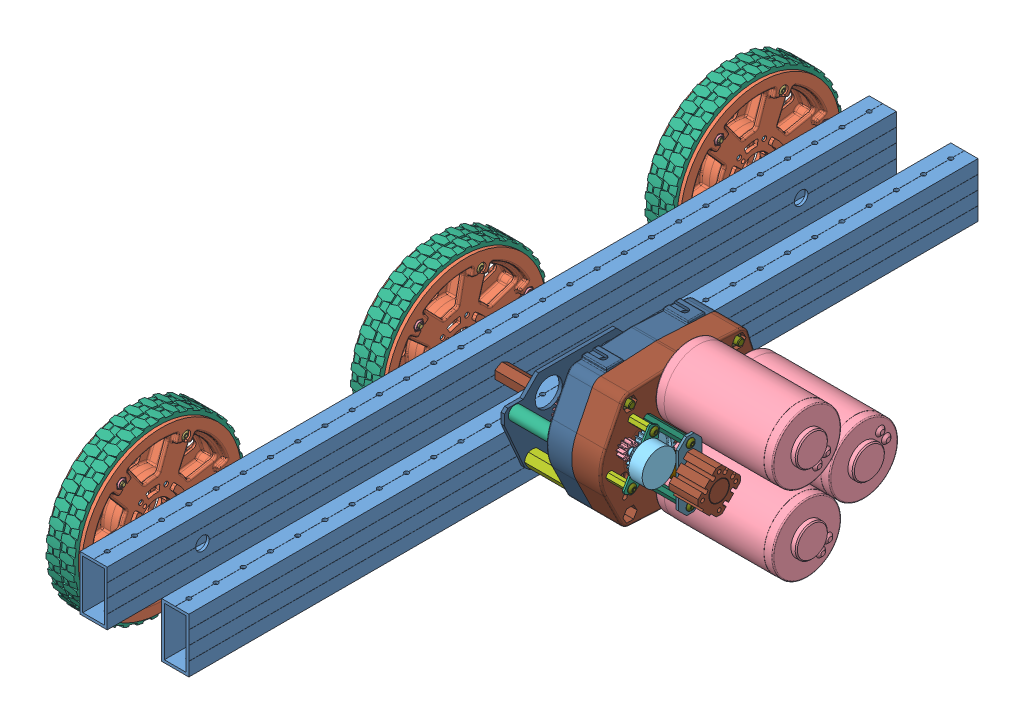
SolidWorks assembly Left Side, Three Wheels, configuration Default. Lengths in mm.
Overall size (675.44 616.63 996.85).
195 component instances, 70 part files, 12 mates.
Components (placement in the parent):
- Base Side Rail-1: Base Side Rail [Default] at (302.3871 430.5681 230.9701) size (25.4 50.8 762)
- 6 inch Traction Wheel and Tire-1: 6 inch Traction Wheel and Tire [Default] at (365.153 367.9 243.3926) x (0 -0.157312 0.987549) z (-1 0 0) size (172.54 172.54 36.19)
  - 6 inch Traction Wheel-1: 6 inch Traction Wheel [Default] at (78.2207 75.8412 104.0409) size (149.22 149.22 36.2)
    - 217-2589-001 Rev3-1: 217-2589-001 Rev3 [Default] at origin size (149.22 149.22 19.81)
    - 217-2589-001 Rev3-2: 217-2589-001 Rev3 [Default] x (-1 0 0) z (0 0 -1) size (149.22 149.22 19.81)
    - SCREW-832-1250-1: SCREW-832-1250 [Default] at (60.96 0 -15.8623) x (0 0 1) z (-1 0 0) size (33.96 7.92 7.92)
    - NUT-832-NYLOCK-1: NUT-832-NYLOCK [Default] at (60.96 0 12.0688) x (0.866025 0.5 0) z (0.5 -0.866025 0) size (10.2 5.86 8.12)
    - BEAM-0750-1: BEAM-0750 [Default] at (11.9062 -20.6222 0.0635) x (0.866025 0.5 0) z (-0.5 0.866025 0) size (7.33 19.93 6.35)
    - BEAM-0750-2: BEAM-0750 [Default] at (-11.9062 -20.6222 0.0635) x (0.866025 -0.5 0) z (0.5 0.866025 0) size (7.33 19.93 6.35)
    - BEAM-0750-3: BEAM-0750 [Default] at (-23.8125 0 0.0635) x (0 -1 0) z (1 0 0) size (7.33 19.93 6.35)
    - BEAM-0750-4: BEAM-0750 [Default] at (-11.9062 20.6222 0.0635) x (-0.866025 -0.5 0) z (0.5 -0.866025 0) size (7.33 19.93 6.35)
    - BEAM-0750-5: BEAM-0750 [Default] at (11.9062 20.6222 0.0635) x (-0.866025 0.5 0) z (-0.5 -0.866025 0) size (7.33 19.93 6.35)
    - BEAM-0750-6: BEAM-0750 [Default] at (23.8125 0 0.0635) x (0 1 0) z (-1 0 0) size (7.33 19.93 6.35)
    - SCREW-832-1250-2: SCREW-832-1250 [Default] at (30.48 52.7929 15.8623) x (0 0 -1) z (0.923728 0.383049 0) size (33.96 7.92 7.92)
    - NUT-832-NYLOCK-2: NUT-832-NYLOCK [Default] at (30.48 52.7929 -12.0688) x (-0.866025 -0.5 0) z (0.5 -0.866025 0) size (10.2 5.86 8.12)
    - NUT-832-NYLOCK-3: NUT-832-NYLOCK [Default] at (30.48 -52.7929 -12.0688) x (0 1 0) z (-1 0 0) size (10.2 5.86 8.12)
    - NUT-832-NYLOCK-4: NUT-832-NYLOCK [Default] at (-60.96 0 -12.0688) x (0.866025 -0.5 0) z (0.5 0.866025 0) size (10.2 5.86 8.12)
    - SCREW-832-1250-3: SCREW-832-1250 [Default] at (-30.48 -52.7929 -15.8623) x (0 0 1) z (0.5 0.866025 0) size (33.96 7.92 7.92)
    - SCREW-832-1250-4: SCREW-832-1250 [Default] at (-30.48 52.7929 -15.8623) x (0 0 1) z (0.5 -0.866025 0) size (33.96 7.92 7.92)
    - NUT-832-NYLOCK-5: NUT-832-NYLOCK [Default] at (-30.48 -52.7929 12.0688) x (0 -1 0) z (-1 0 0) size (10.2 5.86 8.12)
    - NUT-832-NYLOCK-6: NUT-832-NYLOCK [Default] at (-30.48 52.7929 12.0688) x (-0.866025 0.5 0) z (0.5 0.866025 0) size (10.2 5.86 8.12)
    - SCREW-832-1250-5: SCREW-832-1250 [Default] at (30.48 -52.7929 15.8623) x (0 0 -1) z (-0.130134 -0.991496 0) size (33.96 7.92 7.92)
    - SCREW-832-1250-6: SCREW-832-1250 [Default] at (-60.96 0 15.8623) x (0 0 -1) z (-0.793594 0.608447 0) size (33.96 7.92 7.92)
  - 6 inch Traction Tire-1: 6 inch Traction Tire [Default] at (78.2207 75.8412 97.6909) x (0.995848 0.091028 0) z (0 0 1) size (158.75 158.75 12.71)
    - 217-2860-001 Rev3-1: 217-2860-001 Rev3 [Default] at origin size (158.75 158.75 12.71)
    - 217-2860-011 Rev1-1: 217-2860-011 Rev1 [Default] at origin size (146.53 146.53 8.05)
  - 6 inch Traction Tire-2: 6 inch Traction Tire [Default] at (78.2207 75.8412 110.3909) size (158.75 158.75 12.71)
    - 217-2860-001 Rev3-1: 217-2860-001 Rev3 [Default] at origin size (158.75 158.75 12.71)
    - 217-2860-011 Rev1-1: 217-2860-011 Rev1 [Default] at origin size (146.53 146.53 8.05)
- 6 inch Traction Wheel and Tire-2: 6 inch Traction Wheel and Tire [Default] at (365.153 366.208 803.516) x (0 -0.136703 0.990612) z (-1 0 0) size (172.54 172.54 36.19)
  - 6 inch Traction Wheel-1: 6 inch Traction Wheel [Default] at (78.2207 75.8412 104.0409) size (149.22 149.22 36.2)
    - 217-2589-001 Rev3-1: 217-2589-001 Rev3 [Default] at origin size (149.22 149.22 19.81)
    - 217-2589-001 Rev3-2: 217-2589-001 Rev3 [Default] x (-1 0 0) z (0 0 -1) size (149.22 149.22 19.81)
    - SCREW-832-1250-1: SCREW-832-1250 [Default] at (60.96 0 -15.8623) x (0 0 1) z (-1 0 0) size (33.96 7.92 7.92)
    - NUT-832-NYLOCK-1: NUT-832-NYLOCK [Default] at (60.96 0 12.0688) x (0.866025 0.5 0) z (0.5 -0.866025 0) size (10.2 5.86 8.12)
    - BEAM-0750-1: BEAM-0750 [Default] at (11.9062 -20.6222 0.0635) x (0.866025 0.5 0) z (-0.5 0.866025 0) size (7.33 19.93 6.35)
    - BEAM-0750-2: BEAM-0750 [Default] at (-11.9062 -20.6222 0.0635) x (0.866025 -0.5 0) z (0.5 0.866025 0) size (7.33 19.93 6.35)
    - BEAM-0750-3: BEAM-0750 [Default] at (-23.8125 0 0.0635) x (0 -1 0) z (1 0 0) size (7.33 19.93 6.35)
    - BEAM-0750-4: BEAM-0750 [Default] at (-11.9062 20.6222 0.0635) x (-0.866025 -0.5 0) z (0.5 -0.866025 0) size (7.33 19.93 6.35)
    - BEAM-0750-5: BEAM-0750 [Default] at (11.9062 20.6222 0.0635) x (-0.866025 0.5 0) z (-0.5 -0.866025 0) size (7.33 19.93 6.35)
    - BEAM-0750-6: BEAM-0750 [Default] at (23.8125 0 0.0635) x (0 1 0) z (-1 0 0) size (7.33 19.93 6.35)
    - SCREW-832-1250-2: SCREW-832-1250 [Default] at (30.48 52.7929 15.8623) x (0 0 -1) z (0.923728 0.383049 0) size (33.96 7.92 7.92)
    - NUT-832-NYLOCK-2: NUT-832-NYLOCK [Default] at (30.48 52.7929 -12.0688) x (-0.866025 -0.5 0) z (0.5 -0.866025 0) size (10.2 5.86 8.12)
    - NUT-832-NYLOCK-3: NUT-832-NYLOCK [Default] at (30.48 -52.7929 -12.0688) x (0 1 0) z (-1 0 0) size (10.2 5.86 8.12)
    - NUT-832-NYLOCK-4: NUT-832-NYLOCK [Default] at (-60.96 0 -12.0688) x (0.866025 -0.5 0) z (0.5 0.866025 0) size (10.2 5.86 8.12)
    - SCREW-832-1250-3: SCREW-832-1250 [Default] at (-30.48 -52.7929 -15.8623) x (0 0 1) z (0.5 0.866025 0) size (33.96 7.92 7.92)
    - SCREW-832-1250-4: SCREW-832-1250 [Default] at (-30.48 52.7929 -15.8623) x (0 0 1) z (0.5 -0.866025 0) size (33.96 7.92 7.92)
    - NUT-832-NYLOCK-5: NUT-832-NYLOCK [Default] at (-30.48 -52.7929 12.0688) x (0 -1 0) z (-1 0 0) size (10.2 5.86 8.12)
    - NUT-832-NYLOCK-6: NUT-832-NYLOCK [Default] at (-30.48 52.7929 12.0688) x (-0.866025 0.5 0) z (0.5 0.866025 0) size (10.2 5.86 8.12)
    - SCREW-832-1250-5: SCREW-832-1250 [Default] at (30.48 -52.7929 15.8623) x (0 0 -1) z (-0.130134 -0.991496 0) size (33.96 7.92 7.92)
    - SCREW-832-1250-6: SCREW-832-1250 [Default] at (-60.96 0 15.8623) x (0 0 -1) z (-0.793594 0.608447 0) size (33.96 7.92 7.92)
  - 6 inch Traction Tire-1: 6 inch Traction Tire [Default] at (78.2207 75.8412 97.6909) x (0.995848 0.091028 0) z (0 0 1) size (158.75 158.75 12.71)
    - 217-2860-001 Rev3-1: 217-2860-001 Rev3 [Default] at origin size (158.75 158.75 12.71)
    - 217-2860-011 Rev1-1: 217-2860-011 Rev1 [Default] at origin size (146.53 146.53 8.05)
  - 6 inch Traction Tire-2: 6 inch Traction Tire [Default] at (78.2207 75.8412 110.3909) size (158.75 158.75 12.71)
    - 217-2860-001 Rev3-1: 217-2860-001 Rev3 [Default] at origin size (158.75 158.75 12.71)
    - 217-2860-011 Rev1-1: 217-2860-011 Rev1 [Default] at origin size (146.53 146.53 8.05)
- 6 inch Traction Wheel and Tire-3: 6 inch Traction Wheel and Tire [Default] at (369.9155 379.6254 515.6219) x (0 -0.280392 0.959885) z (-1 0 0) size (172.54 172.54 36.19)
  - 6 inch Traction Wheel-1: 6 inch Traction Wheel [Default] at (78.2207 75.8412 104.0409) size (149.22 149.22 36.2)
    - 217-2589-001 Rev3-1: 217-2589-001 Rev3 [Default] at origin size (149.22 149.22 19.81)
    - 217-2589-001 Rev3-2: 217-2589-001 Rev3 [Default] x (-1 0 0) z (0 0 -1) size (149.22 149.22 19.81)
    - SCREW-832-1250-1: SCREW-832-1250 [Default] at (60.96 0 -15.8623) x (0 0 1) z (-1 0 0) size (33.96 7.92 7.92)
    - NUT-832-NYLOCK-1: NUT-832-NYLOCK [Default] at (60.96 0 12.0688) x (0.866025 0.5 0) z (0.5 -0.866025 0) size (10.2 5.86 8.12)
    - BEAM-0750-1: BEAM-0750 [Default] at (11.9062 -20.6222 0.0635) x (0.866025 0.5 0) z (-0.5 0.866025 0) size (7.33 19.93 6.35)
    - BEAM-0750-2: BEAM-0750 [Default] at (-11.9062 -20.6222 0.0635) x (0.866025 -0.5 0) z (0.5 0.866025 0) size (7.33 19.93 6.35)
    - BEAM-0750-3: BEAM-0750 [Default] at (-23.8125 0 0.0635) x (0 -1 0) z (1 0 0) size (7.33 19.93 6.35)
    - BEAM-0750-4: BEAM-0750 [Default] at (-11.9062 20.6222 0.0635) x (-0.866025 -0.5 0) z (0.5 -0.866025 0) size (7.33 19.93 6.35)
    - BEAM-0750-5: BEAM-0750 [Default] at (11.9062 20.6222 0.0635) x (-0.866025 0.5 0) z (-0.5 -0.866025 0) size (7.33 19.93 6.35)
    - BEAM-0750-6: BEAM-0750 [Default] at (23.8125 0 0.0635) x (0 1 0) z (-1 0 0) size (7.33 19.93 6.35)
    - SCREW-832-1250-2: SCREW-832-1250 [Default] at (30.48 52.7929 15.8623) x (0 0 -1) z (0.923728 0.383049 0) size (33.96 7.92 7.92)
    - NUT-832-NYLOCK-2: NUT-832-NYLOCK [Default] at (30.48 52.7929 -12.0688) x (-0.866025 -0.5 0) z (0.5 -0.866025 0) size (10.2 5.86 8.12)
    - NUT-832-NYLOCK-3: NUT-832-NYLOCK [Default] at (30.48 -52.7929 -12.0688) x (0 1 0) z (-1 0 0) size (10.2 5.86 8.12)
    - NUT-832-NYLOCK-4: NUT-832-NYLOCK [Default] at (-60.96 0 -12.0688) x (0.866025 -0.5 0) z (0.5 0.866025 0) size (10.2 5.86 8.12)
    - SCREW-832-1250-3: SCREW-832-1250 [Default] at (-30.48 -52.7929 -15.8623) x (0 0 1) z (0.5 0.866025 0) size (33.96 7.92 7.92)
    - SCREW-832-1250-4: SCREW-832-1250 [Default] at (-30.48 52.7929 -15.8623) x (0 0 1) z (0.5 -0.866025 0) size (33.96 7.92 7.92)
    - NUT-832-NYLOCK-5: NUT-832-NYLOCK [Default] at (-30.48 -52.7929 12.0688) x (0 -1 0) z (-1 0 0) size (10.2 5.86 8.12)
    - NUT-832-NYLOCK-6: NUT-832-NYLOCK [Default] at (-30.48 52.7929 12.0688) x (-0.866025 0.5 0) z (0.5 0.866025 0) size (10.2 5.86 8.12)
    - SCREW-832-1250-5: SCREW-832-1250 [Default] at (30.48 -52.7929 15.8623) x (0 0 -1) z (-0.130134 -0.991496 0) size (33.96 7.92 7.92)
    - SCREW-832-1250-6: SCREW-832-1250 [Default] at (-60.96 0 15.8623) x (0 0 -1) z (-0.793594 0.608447 0) size (33.96 7.92 7.92)
  - 6 inch Traction Tire-1: 6 inch Traction Tire [Default] at (78.2207 75.8412 97.6909) x (0.995848 0.091028 0) z (0 0 1) size (158.75 158.75 12.71)
    - 217-2860-001 Rev3-1: 217-2860-001 Rev3 [Default] at origin size (158.75 158.75 12.71)
    - 217-2860-011 Rev1-1: 217-2860-011 Rev1 [Default] at origin size (146.53 146.53 8.05)
  - 6 inch Traction Tire-2: 6 inch Traction Tire [Default] at (78.2207 75.8412 110.3909) size (158.75 158.75 12.71)
    - 217-2860-001 Rev3-1: 217-2860-001 Rev3 [Default] at origin size (158.75 158.75 12.71)
    - 217-2860-011 Rev1-1: 217-2860-011 Rev1 [Default] at origin size (146.53 146.53 8.05)
- Base Side Rail-2: Base Side Rail [Default] at (378.5871 430.5681 230.9701) size (25.4 50.8 762)
- 3 CIM Ball Shifter with WCD Output-1: 3 CIM Ball Shifter with WCD Output [Default] at (486.2323 470.3699 647.5093) x (0 1 0) z (-1 0 0) size (169.11 183.68 312.65)
  - 217-2733-001 Rev2-1: 217-2733-001 Rev2 [Default] at (0 53.4162 37.6682) x (0 0 1) z (-0.00054 -1 0) size (7.11 24.61 24.61)
  - 217-2733-001 Rev2-2: 217-2733-001 Rev2 [Default] at (0 53.4162 7.9248) x (0 0 -1) z (-0.038475 0.99926 0) size (7.11 24.61 24.61)
  - 217-2731-001 Rev2-1: 217-2731-001 Rev2 [Default] at (0 0 0.0381) x (-0.099212 0.995066 0) z (0.995066 0.099212 0) size (31.12 7.94 31.12)
  - 217-2789-001 Rev2-1: 217-2789-001 Rev2 [Default] at (0 0 43.2943) x (0 0 -1) z (-0.58471 0.811243 0) size (11.1 38.4 38.4)
  - 217-2778-001 Rev2_NCQ8A075-050M_1-1: 217-2778-001 Rev2_NCQ8A075-050M_1 [Default] at (0 0 -53.848) x (-0.707107 0.707107 0) z (0 0 1) size (31.75 33.34 39.88)
    - 217-2778-002_075A-1: 217-2778-002_075A [Default] at origin size (31.75 33.34 26.92)
    - 217-2778-003_075M-1: 217-2778-003_075M [Default] at (0 0 -8.85) x (0.866025 -0.5 0) z (0 0 1) size (18.95 18.95 35.27)
    - 217-2778-004_075-1: 217-2778-004_075 [Default] at (0 0 10.362) size (21 20.74 0.97)
  - 217-2428-012 Rev2-1: 217-2428-012 Rev2 [Default] at (0 0 -40.386) size (63.5 22.23 2.29)
  - 217-2428-005 Rev1-1: 217-2428-005 Rev1 [Default] at (25.4 0 -19.05) x (-0.557362 -0.83027 0) z (-0.83027 0.557362 0) size (7.33 38.98 6.35)
  - 217-2428-005 Rev1-2: 217-2428-005 Rev1 [Default] at (-25.4 0 -19.05) x (0.667436 0.744667 0) z (0.744667 -0.667436 0) size (7.33 38.98 6.35)
  - SCREW-832-0375-1: SCREW-832-0375 [Default] at (25.4 0 -42.5958) x (0 0 1) z (-0.875404 0.483392 0) size (11.73 7.92 7.92)
  - SCREW-832-0375-2: SCREW-832-0375 [Default] at (-25.4 0 -42.5958) x (0 0 1) z (-0.966319 0.257347 0) size (11.73 7.92 7.92)
  - SCREW-832-0375-3: SCREW-832-0375 [Default] at (25.4 0 5.3848) x (0 0 -1) z (1 0 0) size (11.73 7.92 7.92)
  - SCREW-832-0375-4: SCREW-832-0375 [Default] at (-25.4 0 5.3848) x (0 0 -1) z (0.941463 -0.337115 0) size (11.73 7.92 7.92)
  - SBS1_SBS-0632-0250-1: SBS1_SBS-0632-0250 [Default] at (15.494 0 -36.2458) x (0 0 -1) z (0.854303 -0.519775 0) size (8.57 6.68 6.65)
  - SBS1_SBS-0632-0250-2: SBS1_SBS-0632-0250 [Default] at (-15.494 0 -36.2458) x (0 0 -1) z (0.854303 -0.519775 0) size (8.57 6.68 6.65)
  - 217-4098-100 Rev1-1: 217-4098-100 Rev1 [Default] at (0 0 -16.927) x (-0.503316 0.864103 0) z (0 0 1) size (18.03 19.79 22.46)
    - 217-4098-006 Rev2-1: 217-4098-006 Rev2 [Default] at (0 0 -4.6312) x (0 -1 0) z (0 0 -1) size (18.09 11.02 22.46)
    - 217-4098-006 Rev2-2: 217-4098-006 Rev2 [Default] at (0 0 -4.6312) x (0 1 0) z (0 0 -1) size (18.09 11.02 22.46)
    - 217-3489-001 Rev1-1: 217-3489-001 Rev1 [Default] at (0 0 -4.6312) x (0 0 1) z (-0.980217 -0.197926 0) size (4.77 12.7 12.7)
    - 97633A130_97633A130_grv-1: 97633A130_97633A130_grv [Default] at (0 0 -7.33) x (0 0 -1) z (0.979861 0.199683 0) size (0.64 8.74 7.34)
    - 91251A107_91251A107-1: 91251A107_91251A107 [Default] at (-4.8375 -6.735 -9.4343) x (0 0.863883 -0.503692) z (-1 0 0) size (4.65 4.65 10.79)
    - 91251A107_91251A107-2: 91251A107_91251A107 [Default] at (4.8375 6.735 -9.4343) x (0 0.470889 -0.882193) z (1 0 0) size (4.65 4.65 10.79)
  - 217-2428-017 Rev2-1: 217-2428-017 Rev2 [Default] at (12.7 -21.997 -3.614) x (-0.578458 -0.815712 0) z (0 0 -1) size (14.73 14.73 7.37)
  - 217-2428-016 Rev3_Spur01-1: 217-2428-016 Rev3_Spur01 [Default] at (0 0 -3.614) x (0.873157 -0.48744 0) z (0 0 1) size (40.67 40.74 13.32)
  - 217-2428-019 Rev1-1: 217-2428-019 Rev1 [Default] at (12.7 -21.997 -20.6248) x (0.866025 0.5 0) z (0 0 1) size (50.8 19.05 1.57)
  - 217-2428-006 Rev1-1: 217-2428-006 Rev1 [Default] at (32.079 -14.2875 -9.525) x (-0.752416 0.658689 0) z (0.658689 0.752416 0) size (7.33 19.93 6.35)
  - 217-2428-006 Rev1-2: 217-2428-006 Rev1 [Default] at (-3.6662 -34.925 -9.525) x (0.84498 0.534798 0) z (0.534798 -0.84498 0) size (7.33 19.93 6.35)
  - SCREW-832-0375-5: SCREW-832-0375 [Default] at (32.079 -14.2875 4.7498) x (0 0 -1) z (0.980613 0.195955 0) size (11.73 7.92 7.92)
  - SCREW-832-0375-6: SCREW-832-0375 [Default] at (-3.6662 -34.925 5.3848) x (0 0 -1) z (-0.672515 -0.740083 0) size (11.73 7.92 7.92)
  - SCREW-832-0375-7: SCREW-832-0375 [Default] at (-3.6662 -34.925 -22.8346) x (0 0 1) z (0.948865 0.315681 0) size (11.73 7.92 7.92)
  - SCREW-832-0375-8: SCREW-832-0375 [Default] at (32.079 -14.2875 -22.8346) x (0 0 1) z (-0.875404 0.483392 0) size (11.73 7.92 7.92)
  - 217-2614-001_12t-1: 217-2614-001_12t [Default] at (36.9798 39.6868 15.8623) x (-0.087156 0.996195 0) z (0 0 1) size (18.29 18.29 19)
  - 217-2761-001 rev1-1: 217-2761-001 rev1 [Default] at (33.1943 39.3556 16.1) x (0.087156 -0.996195 0) z (0 0 1) size (2 2 20)
  - 217-2761-001 rev1-2: 217-2761-001 rev1 [Default] at (-40.7653 40.018 16.1) x (0.087156 0.996195 0) z (0 0 1) size (2 2 20)
  - 217-2614-001_12t-2: 217-2614-001_12t [Default] at (-36.9798 39.6868 15.8623) x (0.087156 0.996195 0) z (0 0 1) size (18.29 18.29 19)
  - 217-2614-001_12t-3: 217-2614-001_12t [Default] at (0 92.8624 15.8623) x (0.97459 0.223996 0) z (0 0 1) size (18.29 18.29 19)
  - 217-2761-001 rev1-3: 217-2761-001 rev1 [Default] at (-0.8512 96.5658 16.1) x (0.97459 0.223996 0) z (0 0 1) size (2 2 20)
  - 217-3195-002 rev2-1: 217-3195-002 rev2 [Default] at (0 0 50.546) x (-1 0 0) z (0 0 -1) size (114.31 152.24 24.96)
  - 217-3195-001 Rev1-1: 217-3195-001 Rev1 [Default] at origin size (113.41 152.24 26.86)
  - Nylock Nut_NNY2520-ZC-1: Nylock Nut_NNY2520-ZC [Default] at (48.8823 73.025 37.846) x (0 0.866025 -0.5) z (-1 0 0) size (12.85 11.89 7.62)
  - Nylock Nut_NNY2520-ZC-2: Nylock Nut_NNY2520-ZC [Default] at (48.8823 -3.175 37.846) x (0 0 -1) z (-1 0 0) size (12.85 11.89 7.62)
  - Nylock Nut_NNY2520-ZC-3: Nylock Nut_NNY2520-ZC [Default] at (44.45 85.725 7.8613) x (0 1 0) z (0 0 -1) size (12.85 11.89 7.62)
  - 276-1027-001-1: 276-1027-001 [Default] at (47.625 58.1787 6.35) x (0 1 0) z (-1 0 0) size (8.61 5.64 9.94)
  - 276-1027-001-2: 276-1027-001 [Default] at (-47.625 58.1787 6.35) x (0 -1 0) z (1 0 0) size (8.61 5.64 9.94)
  - SCREW-832-1750-1: SCREW-832-1750 [Default] at (-47.625 58.1787 47.0408) x (0 0 -1) z (-0.960822 -0.277167 0) size (46.66 7.92 7.92)
  - SCREW-832-1750-2: SCREW-832-1750 [Default] at (47.625 58.1787 47.0408) x (0 0 -1) z (-0.960822 -0.277167 0) size (46.66 7.92 7.92)
  - Nylock Nut_NNY2520-ZC-4: Nylock Nut_NNY2520-ZC [Default] at (44.45 -15.875 7.8613) x (0 1 0) z (0 0 -1) size (12.85 11.89 7.62)
  - 217-2428-004 Rev3-1: 217-2428-004 Rev3 [Default] at (0 53.4162 22.7711) x (-0.709585 0.70462 0) z (0 0 1) size (11 9.53 43.92)
  - SBS1_SBS-2520-1625SS-1: SBS1_SBS-2520-1625SS [Default] at (44.45 85.725 42.4688) x (0 0 -1) z (-0.251219 0.96793 0) size (45.3 11.2 11.18)
  - SBS1_SBS-2520-1625SS-2: SBS1_SBS-2520-1625SS [Default] at (44.45 -15.875 42.4688) x (0 0 -1) z (-0.251219 0.96793 0) size (45.3 11.2 11.18)
  - SBS1_SBS2520-1750-1: SBS1_SBS2520-1750 [Default] at (-44.45 85.725 7.4422) x (0 0 1) z (-0.031478 0.999504 0) size (48.48 11.22 11.17)
  - SBS1_SBS2520-1750-2: SBS1_SBS2520-1750 [Default] at (-44.45 -15.875 7.4422) x (0 0 1) z (-0.937114 -0.349025 0) size (48.48 11.22 11.17)
  - 217-2428-021 Rev1-1: 217-2428-021 Rev1 [Default] at (0 53.4162 9.5123) x (0.451333 -0.892356 0) z (0 0 1) size (15.88 15.88 3.17)
  - 217-2428-029 Rev1-1: 217-2428-029 Rev1 [Default] at (0 53.4162 36.957) x (0.999846 0.017557 0) z (0 0 1) size (15.88 15.88 1.12)
  - Grayhill Lock Washer-1: Grayhill Lock Washer [Default] at (12.7 -21.997 -18.6817) x (0.467173 -0.884166 0) z (0 0 1) size (19.69 19.69 0.74)
  - Grayhill Nut-1: Grayhill Nut [Default] at (12.7 -21.997 -17.0434) x (0.984088 0.177684 0) z (0 0 1) size (18.33 15.88 2.54)
  - 217-2000-1: 217-2000 [Default] at (0 92.8624 0) x (0 0 -1) z (0.223996 -0.97459 0) size (150.2 64.01 64.01)
  - 217-2000-2: 217-2000 [Default] at (-36.9798 39.6868 0) x (0 0 -1) z (0.996195 -0.087156 0) size (150.2 64.01 64.01)
  - 217-2000-3: 217-2000 [Default] at (36.9798 39.6868 0) x (0 0 -1) z (0.996195 0.087156 0) size (150.2 64.01 64.01)
  - Grahill Encoder-1: Grahill Encoder [Default] at (12.7 -21.997 -16.1798) x (-0.580071 0.814566 0) z (-0.814566 -0.580071 0) size (31.75 31.12 31.75)
  - 217-3195-009 Rev1_wcd 2-1: 217-3195-009 Rev1_wcd 2 [Default] at (0 85.725 50.546) x (-0.998427 -0.056065 0) z (0 0 1) size (12.7 12.7 41.27)
  - 217-3195-006 Rev1_WCD-1: 217-3195-006 Rev1_WCD [Default] at (-44.45 85.725 44.1452) x (0.5 0.866025 0) z (0 0 1) size (12.7 14.66 47.62)
  - 217-3195-009 Rev1_wcd 2-2: 217-3195-009 Rev1_wcd 2 [Default] at (0 -31.75 50.546) x (0.947633 0.319361 0) z (0 0 1) size (12.7 12.7 41.27)
  - 217-3195-006 Rev1_WCD-2: 217-3195-006 Rev1_WCD [Default] at (-44.45 -15.875 44.1452) x (0.5 -0.866025 0) z (0 0 1) size (12.7 14.66 47.62)
  - Nylock Nut_NNY2520-ZC-5: Nylock Nut_NNY2520-ZC [Default] at (0 -31.75 45.0723) x (-0.5 0.866025 0) z (0 0 -1) size (12.85 11.89 7.62)
  - Nylock Nut_NNY2520-ZC-6: Nylock Nut_NNY2520-ZC [Default] at (0 85.725 45.0723) x (-0.5 0.866025 0) z (0 0 -1) size (12.85 11.89 7.62)
  - SBS1_SBS-2520-2250-1: SBS1_SBS-2520-2250 [Default] at (0 -31.75 98.298) x (0 0 -1) z (-0.933488 -0.358607 0) size (61.18 11.22 11.17)
  - SBS1_SBS2520-0625ZC-1: SBS1_SBS2520-0625ZC [Default] at (-44.45 85.725 98.298) x (0 0 -1) z (0.400817 0.916158 0) size (19.57 11.22 11.17)
  - SBS1_SBS2520-0625ZC-2: SBS1_SBS2520-0625ZC [Default] at (-44.45 -15.875 98.298) x (0 0 -1) z (-0.75178 -0.659414 0) size (19.57 11.22 11.17)
  - SBS1_SBS-2520-2250-2: SBS1_SBS-2520-2250 [Default] at (0 85.725 98.298) x (0 0 -1) z (0.056677 -0.998393 0) size (61.18 11.22 11.17)
  - 217-3195-003 rev2-1: 217-3195-003 rev2 [Default] at (0 0 94.9452) size (88.62 139.7 3.17)
  - 217-2617-003 Rev1-1: 217-2617-003 Rev1 [Default] at (-39.878 35.5392 121.8535) x (-0.5 -0.866025 0) z (0 0 1) size (14.66 12.7 152.4)
  - 217-3109-001 Rev1-1: 217-3109-001 Rev1 [Default] at (-39.878 35.5392 49.1808) x (0 0 1) z (0.312889 -0.94979 0) size (7.94 28.57 28.57)
  - 217-2734-001 Rev3-1: 217-2734-001 Rev3 [Default] at (-39.878 35.5392 98.1202) x (1 0 0) z (0 1 0) size (31.12 7.94 31.12)
  - 217-2617-004 Rev1_97431A340_grv-1: 217-2617-004 Rev1_97431A340_grv [Default] at (-39.878 35.5392 54.8961) x (0 0 1) z (-0.124043 -0.992277 0) size (1.07 20.42 18.58)
  - 217-2617-004 Rev1_97431A340_grv-2: 217-2617-004 Rev1_97431A340_grv [Default] at (0 0 69.215) x (0 0 1) z (-0.124043 -0.992277 0) size (1.07 20.42 18.58)
  - 217-2702-001_20t-1: 217-2702-001_20t [Default] at (0 0 62.357) x (0.998435 0.055929 0) z (0 0 1) size (28.2 28.2 12.65)
  - 217-2715-002 Rev1_64t-1: 217-2715-002 Rev1_64t [Default] at (-39.878 35.5392 61.7541) x (0.866025 -0.5 0) z (0 0 1) size (84.3 84.3 12.65)
  - 217-2704-001_24-1: 217-2704-001_24 [Default] at (0 0 62.357) x (0.450781 0.892635 0) z (0 0 -1) size (33.29 33.29 12.65)
  - 217-2714-002 Rev1_60t-1: 217-2714-002 Rev1_60t [Default] at (-39.878 35.5392 61.7541) x (0.866025 -0.5 0) z (0 0 1) size (78.95 78.95 12.65)
  - 217-3221-002 Rev1-1: 217-3221-002 Rev1 [Default] at (-39.878 35.5392 61.7414) x (0 -1 0) z (0 0 1) size (71.39 71.45 12.62)
  - 217-2705-001_30t-1: 217-2705-001_30t [Default] at (0 0 62.357) x (0.547654 -0.836705 0) z (0 0 1) size (41.01 41.12 12.65)
  - 217-2712-002 Rev1_50t-1: 217-2712-002 Rev1_50t [Default] at (-39.878 35.5392 61.7541) x (0.866025 -0.5 0) z (0 0 1) size (66.7 66.76 12.65)
  - 217-2706-001_34t-1: 217-2706-001_34t [Default] at (0 0 62.357) x (0.998435 0.055929 0) z (0 0 1) size (46.46 46.56 12.65)
  - 217-3288-001 Rev3-1: 217-3288-001 Rev3 [Default] at (0 0 0.0889) x (0.055929 -0.998435 0) z (0 0 1) size (99.51 99.53 98.3)
    - 217-2428-008 Rev2-1: 217-2428-008 Rev2 [Default] at (0 0 10.2679) size (31.75 31.75 1.59)
    - 217-2428-028 Rev1_97633A250-1: 217-2428-028 Rev1_97633A250 [Default] at (0 0 37.1221) x (0 0 1) z (0.9357 -0.352797 0) size (1.07 23.39 21.18)
    - 217-4099-000 Rev2_high gear-1: 217-4099-000 Rev2_high gear [Default] x (-1 0 0) z (0 0 1) size (22.23 22.23 98.3)
      - 217-4098-005 Rev1_91612A226-1: 217-4098-005 Rev1_91612A226 [Default] at (0 0 46.2661) x (-0.144757 0 0.989467) z (0 -1 0) size (3.02 3.15 18.22)
      - 217-4098-003 Rev2-1: 217-4098-003 Rev2 [Default] x (1 0 0) z (0 0 -1) size (22.23 22.23 55.94)
      - 217-4099-002 Rev3-1: 217-4099-002 Rev3 [Default] at (0 0 53.467) x (0 0 1) z (-1 0 0) size (40.96 12.73 14.67)
      - 217-4098-004 Rev1-1: 217-4098-004 Rev1 [Default] at (0 0 14.2494) x (0.393904 0.919152 0) z (0 0 1) size (11.68 11.68 56)
    - 217-2428-007 Rev1-1: 217-2428-007 Rev1 [Default] at (7.809 4.5085 14.2494) x (-0.69071 0.455693 -0.561483) z (-0.67559 -0.683536 0.276329) size (6.35 6.35 6.35)
    - 217-2428-007 Rev1-2: 217-2428-007 Rev1 [Default] at (5.4343 3.1375 26.9494) x (-0.162331 -0.978398 0.128005) z (0.857281 -0.204076 -0.472676) size (6.35 6.35 6.35)
    - 217-3212-101 Rev1-1: 217-3212-101 Rev1 [Default] at (-11.5751 10.4131 45.3224) x (0.923728 0.383049 0) z (0 0 -1) size (46.46 46.56 12.7)
      - 217-2428-022 Rev1-1: 217-2428-022 Rev1 [Default] at (6.7035 14.0527 24.6087) size (28.57 28.57 6.1)
      - 217-3212-001 Rev1_34t-1: 217-3212-001 Rev1_34t [Default] at (6.7035 14.0527 27.9107) size (46.46 46.56 11.11)
    - 217-3222-101 Rev1-1: 217-3222-101 Rev1 [Default] at (21.0941 -5.2804 52.7371) x (-0.889163 -0.457591 0) z (0 0 -1) size (73.87 73.92 12.7)
      - 217-2428-022 Rev1-1: 217-2428-022 Rev1 [Default] at (16.3398 14.3476 19.3234) size (28.57 28.57 6.1)
      - 217-3222-001 Rev1_Spur01-1: 217-3222-001 Rev1_Spur01 [Default] at (16.3398 14.3476 22.6254) x (0.999377 0.0353 0) z (0 0 1) size (71.39 71.45 11.11)
    - 217-2428-007 Rev1-3: 217-2428-007 Rev1 [Default] at (-5.4343 3.1375 26.9494) x (0.928483 0.348617 0.128005) z (-0.251905 0.844465 -0.472676) size (6.35 6.35 6.35)
    - 217-2428-007 Rev1-4: 217-2428-007 Rev1 [Default] at (0 -6.275 26.9494) x (-0.766153 0.629782 0.128005) z (-0.605376 -0.640389 -0.472676) size (6.35 6.35 6.35)
    - 217-2428-007 Rev1-5: 217-2428-007 Rev1 [Default] at (-7.809 4.5085 14.2494) x (-0.049287 -0.826019 -0.561483) z (0.929754 -0.24331 0.276329) size (6.35 6.35 6.35)
    - 217-2428-007 Rev1-6: 217-2428-007 Rev1 [Default] at (0 -9.017 14.2494) x (0.739997 0.370326 -0.561483) z (-0.254164 0.926846 0.276329) size (6.35 6.35 6.35)
  - 217-3210-001 Rev1_30t-1: 217-3210-001 Rev1_30t [Default] at (0 53.4162 30.0736) x (-0.966828 0.255427 0) z (0 0 1) size (41.01 41.12 12.65)
  - 217-2711-002 Rev1_50t-1: 217-2711-002 Rev1_50t [Default] at (0 53.4162 17.4244) x (0.262208 -0.965011 0) z (0 0 1) size (66.7 66.76 12.65)
Mates (geometry in assembly coordinates):
- Distance1: distance = 12.7 mm aligned: plane of Base Side Rail-1 through (289.6871 405.1681 980.2701) normal (-1 0 0); plane of 6 inch Traction Wheel and Tire-1/6 inch Traction Wheel-1/217-2589-001 Rev3-1 through (276.9871 430.4919 332.5701) normal (-1 0 0)
- Distance2: distance = 12.7 mm aligned: plane of Base Side Rail-1 through (289.6871 405.1681 980.2701) normal (-1 0 0); plane of 6 inch Traction Wheel and Tire-3/6 inch Traction Wheel-1/217-2589-001 Rev3-1 through (276.9871 430.4919 611.9701) normal (-1 0 0)
- Distance3: distance = 12.7 mm aligned: plane of Base Side Rail-1 through (289.6871 405.1681 980.2701) normal (-1 0 0); plane of 6 inch Traction Wheel and Tire-2/6 inch Traction Wheel-1/217-2589-001 Rev3-1 through (276.9871 430.6443 891.3701) normal (-1 0 0)
- Concentric1: concentric: cylinder of Base Side Rail-1 through (289.6871 430.6443 891.3701) axis (1 0 0) radius 6.35; cylinder of 6 inch Traction Wheel and Tire-2/6 inch Traction Wheel-1/217-2589-001 Rev3-2 through (224.5996 430.6443 891.3701) axis (1 0 0) radius 14.3
- Concentric2: concentric aligned: cylinder of Base Side Rail-1 through (289.6871 430.4919 611.9701) axis (1 0 0) radius 6.35; cylinder of 6 inch Traction Wheel and Tire-3/6 inch Traction Wheel-1/217-2589-001 Rev3-2 through (254.7621 430.4919 611.9701) axis (1 0 0) radius 14.3
- Concentric3: concentric aligned: cylinder of Base Side Rail-1 through (289.6871 430.4919 332.5701) axis (1 0 0) radius 6.35; cylinder of 6 inch Traction Wheel and Tire-1/6 inch Traction Wheel-1/217-2589-001 Rev3-2 through (249.9996 430.4919 332.5701) axis (1 0 0) radius 14.3
- Coincident1: coincident aligned: plane of Base Side Rail-1 through (289.6871 455.9681 980.2701) normal (0 1 0); plane of Base Side Rail-2 through (365.8871 455.9681 980.2701) normal (0 1 0)
- Coincident2: coincident aligned: plane of Base Side Rail-1 through (302.3871 430.5681 218.2701) normal (0 0 -1); plane of Base Side Rail-2 through (378.5871 430.5681 218.2701) normal (0 0 -1)
- Distance4: distance = 50.8 mm anti-aligned: plane of Base Side Rail-1 through (315.0871 405.1681 980.2701) normal (1 0 0); plane of Base Side Rail-2 through (365.8871 405.1681 980.2701) normal (-1 0 0)
- Concentric4: concentric aligned: cylinder of Base Side Rail-1 through (289.6871 430.4919 611.9701) axis (1 0 0) radius 6.35; cylinder of 3 CIM Ball Shifter with WCD Output-1/217-2734-001 Rev3-1 through (388.1121 430.4919 611.9701) axis (1 0 0) radius 14.2748
- Coincident4: coincident anti-aligned: plane of Base Side Rail-2 through (391.2871 405.1681 980.2701) normal (1 0 0); plane of 3 CIM Ball Shifter with WCD Output-1/217-3195-003 rev2-1 through (391.2871 470.3699 647.5093) normal (-1 0 0)
- Angle1: planar angle = 0 rad aligned: plane of Base Side Rail-2 through (365.8871 455.9681 980.2701) normal (0 1 0); plane of 3 CIM Ball Shifter with WCD Output-1/217-3195-003 rev2-1 through (391.2871 491.0201 584.5681) normal (0 1 0)
